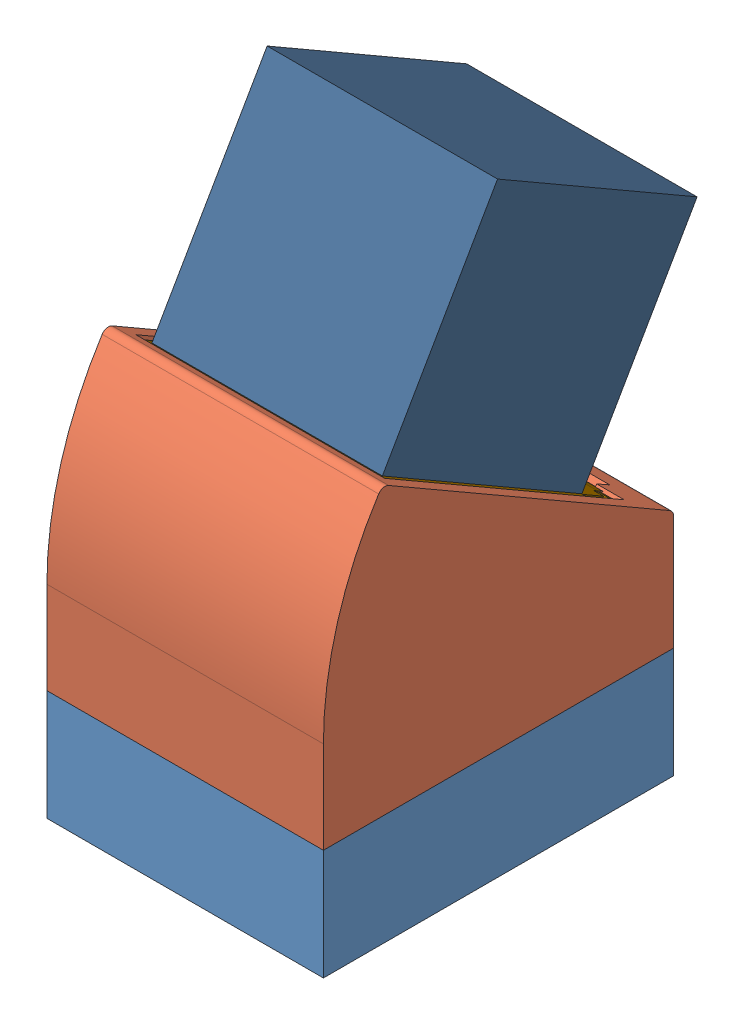
SolidWorks assembly HoloCubic, configuration 默认. Lengths in mm.
Overall size (30 63.52 42.65).
23 component instances, 11 part files, 9 mates.
Components (placement in the parent):
- low-1: low [默认] at (-5.8675 -11.1469 42.5704) size (30 12 38)
- up-1: up [默认] at (-5.8675 0.8531 42.5759) size (30 30.86 38)
- LCD.step-1: LCD.step [默认] at (-18.6101 28.3858 54.9314) x (0 -0.5 -0.866025) z (0 -0.866025 0.5) size (31.51 26.25 5.03)
  - Board.step-1: Board.step [默认] at origin size (29.39 26.24 1.09)
    - Open CASCADE STEP translator 6.8 1.1.1.step-1: Open CASCADE STEP translator 6.8 1.1.1.step [默认] at (0 0 -1.0914) size (29.39 26.24 1.09)
  - R1.step-1: R1.step [默认] at origin size (0.5 1 0.35)
    - 6117106016.step-1: 6117106016.step [默认] at (15.8749 5.4357 0) x (0 1 0) z (0 0 1) size (1 0.5 0.35)
      - Terminal.step-1: Terminal.step [默认] at (-0.5 -0.25 0) size (0.25 0.5 0.35)
        - Open_CASCADE_STEP_translator_6.8_20.2.1.step-1: Open_CASCADE_STEP_translator_6.8_20.2.1.step [默认] at origin size (0.25 0.5 0.35)
      - Terminal.step-2: Terminal.step [默认] at (0.5 0.25 0) x (-1 0 0) z (0 0 1) size (0.25 0.5 0.35)
        - Open_CASCADE_STEP_translator_6.8_20.2.1.step-1: Open_CASCADE_STEP_translator_6.8_20.2.1.step [默认] at origin size (0.25 0.5 0.35)
      - Mid_Body.step-1: Mid_Body.step [默认] at (-0.5 -0.25 0) size (0.93 0.5 0.28)
      - Mark.step-1: Mark.step [默认] at (-0.25 -0.25 0.315) size (0.5 0.5 0.03)
  - Q1.step-1: Q1.step [默认] at origin size (2.9 2.8 1.2)
    - SOT-23-3.step-1: SOT-23-3.step [默认] at (18.2881 5.0545 0) x (-1 0 0) z (0 0 1) size (2.9 2.8 1.2)
  - CON1.step-1: CON1.step [默认] at origin size (5.34 9.5 2.1)
    - fpc.step-1: fpc.step [默认] at (16.7894 13.081 0.0254) x (1 0 0) z (0 0 1) size (5.34 9.5 2.1)
      - ffc_fpc_affc20-16-050-shb-t_(2).step-1: ffc_fpc_affc20-16-050-shb-t_(2).step [默认] at (1.875 2 0) x (0 1 0) z (1 0 0) size (9.5 2.1 5.34)
  - 1.step-1: 1.step [默认] at origin size (31.47 26.24 3.45)
    - tft.step-1: tft.step [默认] at (15.24 12.6239 0.1) x (0 -1 0) z (0 0 -1) size (26.24 31.47 3.45)
      - 1.3_TFT_IPS_-_Flush_Reverse_Mount.step-1: 1.3_TFT_IPS_-_Flush_Reverse_Mount.step [默认] at (-0.503 0.5294 1.6208) size (26.24 31.47 3.45)
- CUBE-1: CUBE [默认] at (-5.4761 24.4715 42.2411) x (1 0 0) z (0 0.5 0.866025) size (25 25 25)
- Main-1: Main [默认] at (7.3904 -7.0555 60.4156) x (0.00013 0 -1) z (0 1 0) size (25 25 6.36)
Mates (geometry in assembly coordinates):
- 平行1: parallel aligned: line of low-1 through (9.1325 0.8531 23.5704) axis (0 0 1); line of up-1 through (9.1325 0.8531 23.5704) axis (0 0 1)
- 平行2: parallel aligned: line of low-1 through (-20.8675 0.8531 61.5704) axis (1 0 0); line of up-1 through (-20.8675 0.8531 61.5704) axis (1 0 0)
- 重合7: coincident anti-aligned: plane of low-1 through (-400005.8675 5.8531 29.5704) normal (0 0 1); plane of Main-1 through (-17.3895 -8.1469 29.5704) normal (0 0 -1)
- 重合8: coincident aligned: line of low-1 through (-20.8675 0.8531 61.5704) axis (1 0 0); line of up-1 through (-20.8675 0.8531 61.5704) axis (1 0 0)
- 重合9: coincident aligned: line of low-1 through (9.1325 0.8531 23.5704) axis (0 0 1); line of up-1 through (9.1325 0.8531 23.5704) axis (0 0 1)
- 重合10: coincident anti-aligned: plane of up-1 through (-400005.8675 145810.5001 252556.9603) normal (0 0.866025 -0.5); plane of LCD.step-1/Board.step-1/Open CASCADE STEP translator 6.8 1.1.1.step-1 through (-18.6101 28.3858 54.9314) normal (0 -0.866025 0.5)
- 重合14: coincident anti-aligned: plane of low-1 through (-5.8675 -8.1469 42.5704) normal (0 1 0); plane of Main-1 through (5.6132 -8.1469 54.5734) normal (0 -1 0)
- 重合15: coincident: point of up-1; point of LCD.step-1/Board.step-1/Open CASCADE STEP translator 6.8 1.1.1.step-1
- 重合16: coincident anti-aligned: plane of LCD.step-1/1.step-1/tft.step-1/1.3_TFT_IPS_-_Flush_Reverse_Mount.step-1 through (-5.4832 23.5899 40.7141) normal (0 0.866025 -0.5); plane of CUBE-1 through (-5.4761 24.4715 42.2411) normal (0 -0.866025 0.5)
